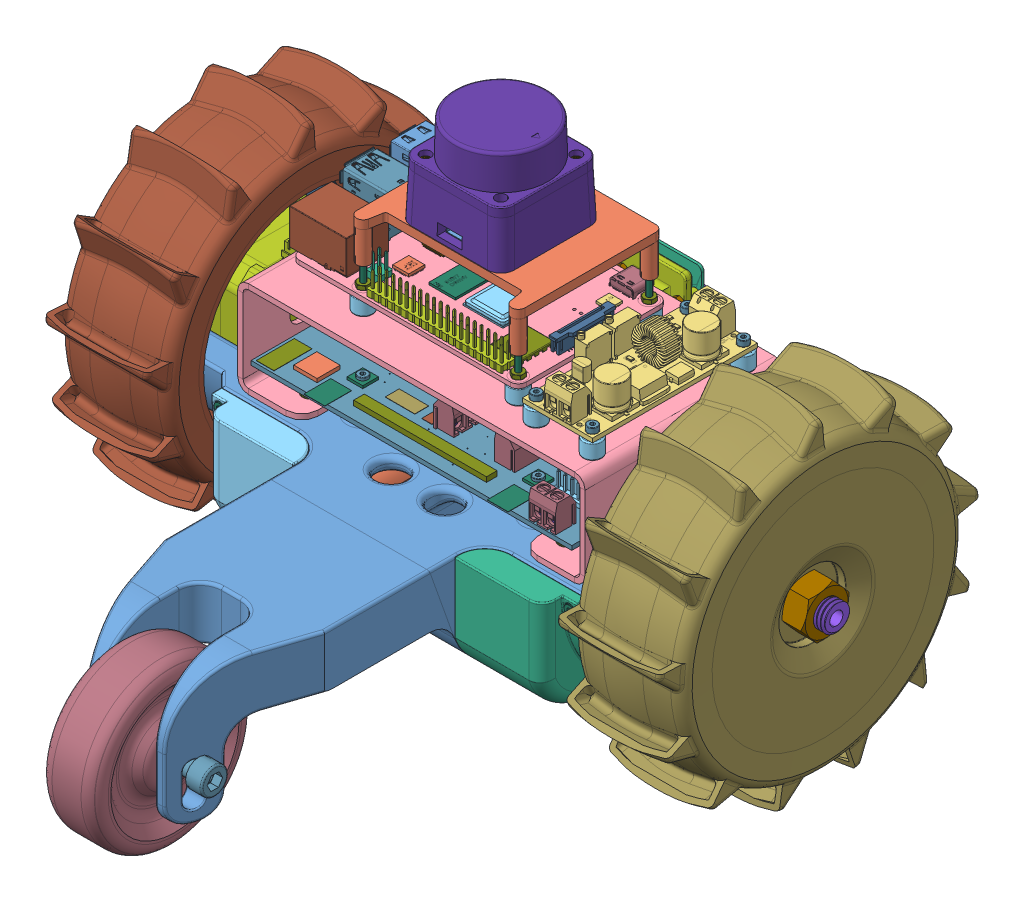
SolidWorks assembly RILey_assembly, configuration Default. Lengths in mm. (continued)
Mates (geometry in assembly coordinates): (continued)
- Width3: width aligned: plane of CameraMountBase-1 through (-15 21.3863 -20.622) normal (-1 0 0); plane of MiddlepartV1-1 through (15 21.3863 -20.622) normal (1 0 0); plane of CameraMountBase-1 through (61.5 -5 45) normal (-1 0 0); plane of MiddlepartV1-1 through (-61.5 -5 45) normal (1 0 0)
- Coincident33: coincident aligned: plane of DRV 8825 With Headers Assem-2/PCB-1 through (-15.9139 22.4151 10.2324) normal (0 1 0); plane of GY-91_MPU9250+BMP280 - Pins Down-1/GY-91 Base-1 through (23.0777 22.4151 10.2748) normal (0 1 0)
- Concentric20: concentric anti-aligned: cylinder of MiddlepartV1-1 through (-106.8137 0 0) axis (1 0 0) radius 4; cylinder of Nema 17_Slim-1 through (113.5 0 0) axis (-1 0 0) radius 2.5
- Concentric21: concentric anti-aligned: cylinder of socket head cap screw 4762_din-9 through (135.25 15.5 15.5) axis (1 0 0) radius 1.5; cylinder of Nema 17_Slim-1 through (95.5 15.5 15.5) axis (-1 0 0) radius 1.2645
- Coincident35: coincident anti-aligned: plane of MiddlepartV1-1 through (95.5 40 -40) normal (-1 0 0); plane of Nema 17_Slim-1 through (95.5 0 0) normal (1 0 0)
- Concentric22: concentric anti-aligned: cylinder of MiddlepartV1-1 through (-84.1863 0 0) axis (-1 0 0) radius 4; cylinder of Nema 17_Slim-2 through (-113.5 0 0) axis (1 0 0) radius 2.5
- Concentric23: concentric anti-aligned: cylinder of socket head cap screw 4762_din-3 through (-135.25 15.5 -15.5) axis (-1 0 0) radius 1.5; cylinder of Nema 17_Slim-2 through (-95.5 15.5 -15.5) axis (1 0 0) radius 1.2645
- Coincident36: coincident anti-aligned: plane of MiddlepartV1-1 through (-95.5 40 -40) normal (1 0 0); plane of Nema 17_Slim-2 through (-95.5 0 0) normal (-1 0 0)
- Distance1: distance = 155 mm anti-aligned: plane of wiel-1 through (75.1265 0 0) normal (-1 0 0); plane of wiel-2 through (71.8138 0 0) normal (-1 0 0)
- Concentric24: concentric anti-aligned: cylinder of wiel-1 through (85.7417 0 0) axis (1 0 0) radius 6.5; cylinder of Nema 17_Slim-1 through (113.5 0 0) axis (-1 0 0) radius 2.5
- Tangent5: tangent aligned: cylinder of MiddlepartV1-1 through (100.5 0 0) axis (-1 0 0) radius 40; plane of CameraMountBase-1 through (15 21.3863 -30) normal (0 0 -1)
- Tangent8: tangent anti-aligned: cylinder of 3_battery_pack-2/Li-ion Battery-1 through (14 -23 -26.7134) axis (0 0 -1) radius 9; plane of MiddlepartV1-1 through (-61.5 -32 45) normal (0 1 0)
- Width4: width anti-aligned: plane of MiddlepartV1-1 through (-2 0 0) normal (-1 0 0); plane of TimeOfFlightMount-1 through (2 0 0) normal (1 0 0); plane of MiddlepartV1-1 through (-5 -10.7713 -54.3331) normal (-0.984808 0.082851 0.152609); plane of TimeOfFlightMount-1 through (5 -10.7713 -54.3331) normal (0.984808 0.082851 0.152609)
- Coincident44: coincident anti-aligned: plane of MiddlepartV1-1 through (0 0 0) normal (0 1 0); plane of 3thFloor-1 through (0 0 0) normal (0 -1 0)
- Concentric31: concentric aligned: cylinder of MiddlepartV1-1 through (48 -9.9497 -27.5) axis (0 1 0) radius 1.75; cylinder of 3thFloor-1 through (48 -4.9497 -27.5) axis (0 1 0) radius 1.75
- Concentric32: concentric aligned: cylinder of MiddlepartV1-1 through (-48 -9.9497 -27.5) axis (0 1 0) radius 1.75; cylinder of 3thFloor-1 through (-48 -4.9497 -27.5) axis (0 1 0) radius 1.75
- Concentric37: concentric aligned: cylinder of 3thFloor-1 through (48 -4.9497 -27.5) axis (0 1 0) radius 1.75; cylinder of socket head cap screw 4762_din-11 through (48 37.75 -27.5) axis (0 1 0) radius 2.75
- Coincident47: coincident anti-aligned: plane of 3thFloor-1 through (41 3 37.5) normal (0 1 0); plane of socket head cap screw 4762_din-11 through (50.75 3 -27.5) normal (0 -1 0)
- Concentric38: concentric aligned: cylinder of 3thFloor-1 through (48 -4.9497 27.5) axis (0 1 0) radius 1.75; cylinder of socket head cap screw 4762_din-12 through (48 37.75 27.5) axis (0 1 0) radius 2.75
- Coincident48: coincident anti-aligned: plane of 3thFloor-1 through (41 3 37.5) normal (0 1 0); plane of socket head cap screw 4762_din-12 through (50.75 3 27.5) normal (0 -1 0)
- Concentric39: concentric aligned: cylinder of 3thFloor-1 through (-48 -4.9497 -27.5) axis (0 1 0) radius 1.75; cylinder of socket head cap screw 4762_din-13 through (-48 37.75 -27.5) axis (0 1 0) radius 2.75
- Coincident49: coincident anti-aligned: plane of 3thFloor-1 through (-41 3 37.5) normal (0 1 0); plane of socket head cap screw 4762_din-13 through (-45.25 3 -27.5) normal (0 -1 0)
- Concentric40: concentric aligned: cylinder of 3thFloor-1 through (-48 -4.9497 27.5) axis (0 1 0) radius 1.75; cylinder of socket head cap screw 4762_din-14 through (-48 37.75 27.5) axis (0 1 0) radius 2.75
- Coincident50: coincident anti-aligned: plane of 3thFloor-1 through (-41 3 37.5) normal (0 1 0); plane of socket head cap screw 4762_din-14 through (-45.25 3 27.5) normal (0 -1 0)
- Concentric41: concentric aligned: cylinder of socket head cap screw 4762_din-12 through (48 37.75 27.5) axis (0 1 0) radius 1.5; cylinder of hex nut style 1 gradeab_din-2 through (48 -30.234 27.5) axis (0 1 0) radius 1.5
- Concentric42: concentric anti-aligned: cylinder of MiddlepartV1-1 through (48 -9.9497 -27.5) axis (0 1 0) radius 1.75; cylinder of hex nut style 1 gradeab_din-3 through (48 17.6375 -27.5) axis (0 -1 0) radius 1.5
- Coincident51: coincident anti-aligned: plane of MiddlepartV1-1 through (-61.5 -5 45) normal (0 -1 0); plane of hex nut style 1 gradeab_din-3 through (48 -5 -24.3246) normal (0 1 0)
- Concentric43: concentric anti-aligned: cylinder of MiddlepartV1-1 through (-48 -9.9497 27.5) axis (0 1 0) radius 1.75; cylinder of hex nut style 1 gradeab_din-4 through (-48 17.6375 27.5) axis (0 -1 0) radius 1.5
- Coincident52: coincident anti-aligned: plane of MiddlepartV1-1 through (-61.5 -5 45) normal (0 -1 0); plane of hex nut style 1 gradeab_din-4 through (-48 -5 30.6754) normal (0 1 0)
- Concentric44: concentric anti-aligned: cylinder of MiddlepartV1-1 through (-48 -9.9497 -27.5) axis (0 1 0) radius 1.75; cylinder of hex nut style 1 gradeab_din-5 through (-48 17.6375 -27.5) axis (0 -1 0) radius 1.5
- Coincident53: coincident anti-aligned: plane of MiddlepartV1-1 through (-61.5 -5 45) normal (0 -1 0); plane of hex nut style 1 gradeab_din-5 through (-48 -5 -24.3246) normal (0 1 0)
- Concentric47: concentric aligned: cylinder of wiel-1 through (116.1265 0 0) axis (-1 0 0) radius 55.5; cylinder of socket head cap screw 4762_din-16 through (61.9923 0 0) axis (-1 0 0) radius 1.9
- Concentric59: concentric anti-aligned: cylinder of Nema 17_Slim-2 through (-113.5 0 0) axis (1 0 0) radius 2.5; cylinder of ReelyBuggyWheel-1 through (-163.278 0 0) axis (-1 0 0) radius 5.75
- Concentric60: concentric anti-aligned: cylinder of Nema 17_Slim-1 through (113.5 0 0) axis (-1 0 0) radius 2.5; cylinder of wiel-2 through (82.429 0 0) axis (1 0 0) radius 6.5
- Concentric61: concentric anti-aligned: cylinder of Nema 17_Slim-1 through (113.5 0 0) axis (-1 0 0) radius 2.5; cylinder of ReelyBuggyWheel_Left-1 through (106.7689 0 0) axis (1 0 0) radius 5.75
- Concentric62: concentric anti-aligned: cylinder of Nema 17_Slim-2 through (-113.5 0 0) axis (1 0 0) radius 2.5; cylinder of ReelyBuggyWheel_Right-1 through (-106.7689 0 0) axis (-1 0 0) radius 5.75
- Distance2: distance = 155 mm anti-aligned: cone of ReelyBuggyWheel_Left-1 through (75.7689 0 0) axis (1 0 0); cone of ReelyBuggyWheel_Right-1 through (-75.7689 0 0) axis (-1 0 0)
- Width7: width aligned: plane of ReelyBuggyWheel_Left-1 through (102.2689 0 0) normal (-1 0 0); plane of ReelyBuggyWheel_Right-1 through (-102.2689 0 0) normal (1 0 0); plane of MiddlepartV1-1 through (-100.5 0 0) normal (-1 0 0); plane of MiddlepartV1-1 through (100.5 0 0) normal (1 0 0)
- Concentric63: concentric anti-aligned: cylinder of Nema 17_Slim-2 through (-113.5 0 0) axis (1 0 0) radius 2.5; cylinder of ReelyBuggyWheel_Left-2 through (-106.5 0 0) axis (-1 0 0) radius 5.75
- Concentric64: concentric anti-aligned: cylinder of Nema 17_Slim-1 through (113.5 0 0) axis (-1 0 0) radius 2.5; cylinder of ReelyBuggyWheel_Right-2 through (106.5 0 0) axis (1 0 0) radius 5.75
- Concentric65: concentric aligned: cylinder of CameraMount-1 through (-8.25 3.5 -37) axis (1 0 0) radius 1.75; cylinder of socket head cap screw 4762_din-29 through (38.75 3.5 -37) axis (1 0 0) radius 1.9
- Coincident65: coincident anti-aligned: plane of CameraMount-1 through (5 4.049 -57.0786) normal (1 0 0); plane of socket head cap screw 4762_din-29 through (5 2.7745 -35.244) normal (-1 0 0)
- Concentric66: concentric aligned: cylinder of MiddlepartV1-1 through (-5.2527 -1 -43.5) axis (1 0 0) radius 1.15; cylinder of socket head cap screw 4762_din-30 through (38.75 -1 -43.5) axis (1 0 0) radius 1.9
- Concentric68: concentric anti-aligned: cylinder of socket head cap screw 4762_din-30 through (38.75 -1 -43.5) axis (1 0 0) radius 1; cylinder of hex nut style 1 gradeab_din-8 through (18.4375 -1 -43.5) axis (-1 0 0) radius 1
- Concentric71: concentric aligned: cylinder of 3thFloor-1 through (-31 45 -24.5) axis (0 -1 0) radius 1; cylinder of socket head cap screw 4762_din-35 through (-31 1.25 -24.5) axis (0 -1 0) radius 1.9
- Coincident71: coincident anti-aligned: plane of 3thFloor-1 through (0 35 0) normal (0 -1 0); plane of socket head cap screw 4762_din-35 through (-32.9 35 -24.5) normal (0 1 0)
- Concentric72: concentric aligned: cylinder of 3thFloor-1 through (-31 45 24.5) axis (0 -1 0) radius 1; cylinder of socket head cap screw 4762_din-36 through (-31 1.25 24.5) axis (0 -1 0) radius 1.9
- Coincident72: coincident anti-aligned: plane of 3thFloor-1 through (0 35 0) normal (0 -1 0); plane of socket head cap screw 4762_din-36 through (-32.9 35 24.5) normal (0 1 0)
- Concentric73: concentric aligned: cylinder of 3thFloor-1 through (27 45 -24.5) axis (0 -1 0) radius 1; cylinder of socket head cap screw 4762_din-37 through (27 1.25 -24.5) axis (0 -1 0) radius 1.9
- Coincident73: coincident anti-aligned: plane of 3thFloor-1 through (0 35 0) normal (0 -1 0); plane of socket head cap screw 4762_din-37 through (25.1 35 -24.5) normal (0 1 0)
- Concentric74: concentric aligned: cylinder of 3thFloor-1 through (27 45 24.5) axis (0 -1 0) radius 1; cylinder of socket head cap screw 4762_din-38 through (27 1.25 24.5) axis (0 -1 0) radius 1.9
- Coincident74: coincident anti-aligned: plane of 3thFloor-1 through (0 35 0) normal (0 -1 0); plane of socket head cap screw 4762_din-38 through (25.1 35 24.5) normal (0 1 0)
- Concentric75: concentric anti-aligned: cylinder of MiddlepartV1-1 through (-5.2527 3.5 -37) axis (1 0 0) radius 1.15; cylinder of CameraMount-1 through (5 3.5 -37) axis (-1 0 0) radius 1
- Coincident75: coincident anti-aligned: plane of Cam V2.1 v1.step-1 through (0 17.1066 -58.9285) normal (0 0.064849 0.997895); plane of CameraMount-1 through (-10.5 19.6013 -59.0906) normal (0 -0.064849 -0.997895)
- Width10: width anti-aligned: plane of CameraMount-1 through (2.25 1.6736 -18.8433) normal (-1 0 0); plane of MiddlepartV1-1 through (-2.25 1.6736 -18.8433) normal (1 0 0); plane of CameraMount-1 through (2 0 0) normal (1 0 0); plane of MiddlepartV1-1 through (-2 0 0) normal (-1 0 0)
- Concentric78: concentric aligned: cylinder of Cam V2.1 v1.step-1 through (10.5 7.1277 -58.28) axis (0 -0.064849 -0.997895) radius 1; cylinder of CameraMount-1 through (10.5 7.9707 -45.3074) axis (0 -0.064849 -0.997895) radius 1.25
- Concentric79: concentric aligned: cylinder of Cam V2.1 v1.step-1 through (-10.5 7.1277 -58.28) axis (0 -0.064849 -0.997895) radius 1; cylinder of CameraMount-1 through (-10.5 7.9707 -45.3074) axis (0 -0.064849 -0.997895) radius 1.25
- Width11: width anti-aligned: plane of Backwheel-1 through (-10.5 -32.6496 136.5106) normal (-1 0 0); plane of MiddlepartV1-2 through (10.5 -32.6496 136.5106) normal (1 0 0); plane of Backwheel-1 through (-11.5 0 105) normal (1 0 0); plane of MiddlepartV1-2 through (11.5 0 105) normal (-1 0 0)
- Tangent10: tangent aligned: cylinder of MiddlepartV1-2 through (35.6484 -32.5 136.5) axis (-1 0 0) radius 3.1; cylinder of Backwheel-1 through (-10.5 -32.6496 136.5106) axis (1 0 0) radius 3.25
- Concentric102: concentric aligned: cylinder of Cam V2.1 v1.step-1 through (-10.5 19.6013 -59.0906) axis (0 -0.064849 -0.997895) radius 1; cylinder of socket head cap screw 4762_din-51 through (-10.5 17.3479 -93.7675) axis (0 -0.064849 -0.997895) radius 1.9
- Coincident99: coincident anti-aligned: plane of Cam V2.1 v1.step-1 through (0 17.0418 -59.9264) normal (0 -0.064849 -0.997895); plane of socket head cap screw 4762_din-51 through (-10.6232 21.4285 -60.2115) normal (0 0.064849 0.997895)
- Concentric103: concentric aligned: cylinder of Cam V2.1 v1.step-1 through (-10.5 7.1277 -58.28) axis (0 -0.064849 -0.997895) radius 1; cylinder of socket head cap screw 4762_din-52 through (-10.5 4.8742 -92.9569) axis (0 -0.064849 -0.997895) radius 1.9
- Coincident100: coincident anti-aligned: plane of Cam V2.1 v1.step-1 through (0 17.0418 -59.9264) normal (0 -0.064849 -0.997895); plane of socket head cap screw 4762_din-52 through (-10.6232 8.9548 -59.4009) normal (0 0.064849 0.997895)
- Concentric104: concentric aligned: cylinder of Cam V2.1 v1.step-1 through (10.5 7.1277 -58.28) axis (0 -0.064849 -0.997895) radius 1; cylinder of socket head cap screw 4762_din-53 through (10.5 4.8742 -92.9569) axis (0 -0.064849 -0.997895) radius 1.9
- Coincident101: coincident anti-aligned: plane of Cam V2.1 v1.step-1 through (0 17.0418 -59.9264) normal (0 -0.064849 -0.997895); plane of socket head cap screw 4762_din-53 through (10.3768 8.9548 -59.4009) normal (0 0.064849 0.997895)
- Concentric105: concentric aligned: cylinder of Cam V2.1 v1.step-1 through (10.5 19.6013 -59.0906) axis (0 -0.064849 -0.997895) radius 1; cylinder of socket head cap screw 4762_din-54 through (10.5 17.3479 -93.7675) axis (0 -0.064849 -0.997895) radius 1.9
- Coincident102: coincident anti-aligned: plane of Cam V2.1 v1.step-1 through (0 17.0418 -59.9264) normal (0 -0.064849 -0.997895); plane of socket head cap screw 4762_din-54 through (10.3768 21.4285 -60.2115) normal (0 0.064849 0.997895)
- Concentric108: concentric anti-aligned: cylinder of MiddlepartV1-1 through (48 -9.9497 -27.5) axis (0 1 0) radius 1.75; cylinder of socket head cap screw 4762_din-58 through (48 -39.75 -27.5) axis (0 -1 0) radius 2.75
- Coincident105: coincident anti-aligned: plane of MiddlepartV1-1 through (-61.5 -5 45) normal (0 -1 0); plane of socket head cap screw 4762_din-58 through (45.25 -5 -27.5) normal (0 1 0)
- Concentric109: concentric anti-aligned: cylinder of MiddlepartV1-1 through (-48 -9.9497 -27.5) axis (0 1 0) radius 1.75; cylinder of socket head cap screw 4762_din-59 through (-48 -39.75 -27.5) axis (0 -1 0) radius 2.75
- Coincident106: coincident anti-aligned: plane of MiddlepartV1-1 through (-61.5 -5 45) normal (0 -1 0); plane of socket head cap screw 4762_din-59 through (-50.75 -5 -27.5) normal (0 1 0)
- Concentric110: concentric anti-aligned: cylinder of MiddlepartV1-1 through (-48 -9.9497 27.5) axis (0 1 0) radius 1.75; cylinder of socket head cap screw 4762_din-61 through (-48 -39.75 27.5) axis (0 -1 0) radius 2.75
- Coincident107: coincident anti-aligned: plane of MiddlepartV1-1 through (-61.5 -5 45) normal (0 -1 0); plane of socket head cap screw 4762_din-61 through (-50.75 -5 27.5) normal (0 1 0)
- Concentric111: concentric anti-aligned: cylinder of MiddlepartV1-1 through (48 -9.9497 27.5) axis (0 1 0) radius 1.75; cylinder of socket head cap screw 4762_din-62 through (48 -39.75 27.5) axis (0 -1 0) radius 2.75
- Coincident108: coincident anti-aligned: plane of MiddlepartV1-1 through (-61.5 -5 45) normal (0 -1 0); plane of socket head cap screw 4762_din-62 through (45.25 -5 27.5) normal (0 1 0)
- Concentric120: concentric: cylinder of Backwheel-1 through (-10.5 -32.6496 136.5106) axis (1 0 0) radius 3.25; cylinder of socket head cap screw 4762_din-64 through (-64.9282 -39.2304 114.5914) axis (-0.948683 0 0.316228) radius 5
- Concentric1211: concentric aligned: cylinder of Backwheel-1 through (-10.5 -32.6496 136.5106) axis (1 0 0) radius 3.25; cylinder of socket head cap screw 4762_din-66 through (57.2465 -32.6496 136.5106) axis (1 0 0) radius 5
- Tangent152: tangent: plane of MiddlepartV1-2 through (30 -97.4342 100) normal (0.948683 0 0.316228); circle of socket head cap screw 4762_din-66
- Concentric122: concentric aligned: cone of socket head cap screw 4762_din-66 through (-25.5035 -32.6496 136.5106) axis (-1 0 0); cylinder of hex nut style 1 gradeab_din-20 through (0.8569 -39.2304 136.65) axis (-1 0 0) radius 3
- Coincident122: coincident: line of MiddlepartV1-1 through (-18.9806 -42.5 133.0581) axis (0 1 0); plane of hex nut style 1 gradeab_din-20 through (-18.9806 -39.2304 126.65) normal (1 0 0)
- Concentric1214: concentric aligned: cylinder of ReelyBuggyWheel_Right-2 through (106.5 0 0) axis (1 0 0) radius 5.75; cylinder of hex nut style 1 gradeab_iso-2 through (92.8625 0 0) axis (1 0 0) radius 5
- Coincident131: coincident anti-aligned: plane of ReelyBuggyWheel_Right-2 through (109.5 0 0) normal (1 0 0); plane of hex nut style 1 gradeab_iso-2 through (109.5 0 16) normal (-1 0 0)
- Concentric1215: concentric aligned: cylinder of ReelyBuggyWheel_Left-2 through (-106.5 0 0) axis (-1 0 0) radius 5.75; cylinder of hex nut style 1 gradeab_iso-3 through (-92.8625 0 0) axis (-1 0 0) radius 5
- Coincident132: coincident anti-aligned: plane of ReelyBuggyWheel_Left-2 through (-109.5 0 0) normal (-1 0 0); plane of hex nut style 1 gradeab_iso-3 through (-109.5 -2.0616 -15.8666) normal (1 0 0)
- Width12: width aligned: plane of 3_battery_pack-1/link2-2 through (-10 -24.5 -26.9134) normal (1 0 0); plane of MiddlepartV1-1 through (-54 -21.5 -26.9134) normal (-1 0 0); plane of 3_battery_pack-1/link2-2 through (-61.5 -5 45) normal (1 0 0); plane of MiddlepartV1-1 through (-2.5 0 0) normal (-1 0 0)
- Tangent12: tangent anti-aligned: plane of MiddlepartV1-1 through (-61.5 -32 45) normal (0 1 0); cylinder of 3_battery_pack-2/Li-ion Battery-3 through (50 -23 -26.7134) axis (0 0 -1) radius 9
- Coincident138: coincident aligned: plane of 3_battery_pack-1/link2-2 through (-11 -24.5 -26.9134) normal (0 0 -1); plane of 3_battery_pack-2/link2-2 through (53 -24.5 -26.9134) normal (0 0 -1)
- Width13: width anti-aligned: plane of 3_battery_pack-2/link2-2 through (10 -21.5 -26.9134) normal (-1 0 0); plane of 3_battery_pack-2/link2-2 through (54 -24.5 -26.9134) normal (1 0 0); plane of MiddlepartV1-1 through (2.5 0 0) normal (1 0 0); plane of MiddlepartV1-1 through (61.5 -5 45) normal (-1 0 0)
- Concentric1220: concentric aligned: cylinder of Nema 17_Slim-2 through (-113.5 0 0) axis (1 0 0) radius 2.5; cylinder of hex screw gradeab fine_iso-1 through (-100.5 0 0) axis (1 0 0) radius 5
- Coincident139: coincident anti-aligned: plane of MiddlepartV1-1 through (-100.5 0 0) normal (-1 0 0); plane of hex screw gradeab fine_iso-1 through (-100.5 -2.768 8.8132) normal (1 0 0)
- Parallel6: parallel anti-aligned: plane of ReelyBuggyWheel_Left-2 through (-106.5 8.4437 -4.875) normal (0 -1 0); plane of hex screw gradeab fine_iso-1 through (-106.9 6.2484 6.8037) normal (0 0.954052 0.299641)
- Coincident141: coincident anti-aligned: plane of ReelyBuggyWheel_Left-2 through (-106.5 0 0) normal (1 0 0); plane of hex screw gradeab fine_iso-1 through (-106.9 -2.768 8.8132) normal (-1 0 0)
- Coincident142: coincident anti-aligned: plane of MiddlepartV1-1 through (100.5 0 0) normal (1 0 0); plane of hex screw gradeab fine_iso-2 through (100.5 9.2376 0) normal (-1 0 0)
- Concentric1222: concentric aligned: cylinder of Nema 17_Slim-1 through (113.5 0 0) axis (-1 0 0) radius 2.5; cylinder of hex screw gradeab fine_iso-2 through (100.5 0 0) axis (-1 0 0) radius 5
- Parallel7: parallel anti-aligned: plane of ReelyBuggyWheel_Right-2 through (106.5 8.4437 4.875) normal (0 -1 0); plane of hex screw gradeab fine_iso-2 through (106.9 9.2376 0) normal (0 0.866025 0.5)
- Coincident144: coincident anti-aligned: plane of ReelyBuggyWheel_Right-2 through (106.5 0 0) normal (-1 0 0); plane of hex screw gradeab fine_iso-2 through (106.9 9.2376 0) normal (1 0 0)
- Concentric1224: concentric anti-aligned: cylinder of MiddlepartV1-1 through (100.5 0 0) axis (-1 0 0) radius 40; cylinder of BatteryCoverFront-1 through (-68.5 0 0) axis (1 0 0) radius 40
- Concentric1225: concentric aligned: cylinder of MiddlepartV1-1 through (-65.5 -3.5 -50) axis (0 0 1) radius 1; cylinder of BatteryCoverFront-1 through (-65.5 -3.5 -44) axis (0 0 1) radius 1
- Concentric1226: concentric aligned: cylinder of MiddlepartV1-1 through (65.5 -3.5 -50) axis (0 0 1) radius 1; cylinder of BatteryCoverFront-1 through (65.5 -3.5 -44) axis (0 0 1) radius 1
- Concentric1229: concentric anti-aligned: cylinder of MiddlepartV1-1 through (65.5 -3.5 -50) axis (0 0 1) radius 1; cylinder of socket head cap screw_iso-9 through (65.5 -3.5 -75.75) axis (0 0 -1) radius 1
- Concentric1231: concentric anti-aligned: cylinder of MiddlepartV1-1 through (-65.5 -3.5 -50) axis (0 0 1) radius 1; cylinder of socket head cap screw_iso-13 through (-65.5 -3.5 -75.75) axis (0 0 -1) radius 1
- Concentric1232: concentric anti-aligned: cylinder of MiddlepartV1-1 through (-65.5 -36.5 -25) axis (0 0 1) radius 1; cylinder of socket head cap screw_iso-15 through (-65.5 -36.5 -55.75) axis (0 0 -1) radius 1
- Concentric1233: concentric anti-aligned: cylinder of MiddlepartV1-1 through (0 -36.5 -25) axis (0 0 1) radius 1; cylinder of socket head cap screw_iso-17 through (0 -36.5 -55.75) axis (0 0 -1) radius 1
- Concentric1234: concentric anti-aligned: cylinder of MiddlepartV1-1 through (65.5 -36.5 -25) axis (0 0 1) radius 1; cylinder of socket head cap screw_iso-16 through (65.5 -36.5 -55.75) axis (0 0 -1) radius 1
- Concentric1246: concentric anti-aligned: cylinder of MiddlepartV1-1 through (-32.85 10 22.85) axis (0 -1 0) radius 1; cylinder of RILey_PCB-1/RILey_PCB.step-1/PCB Component.step-1/Board.step-1 through (-32.85 10 22.85) axis (0 1 0) radius 1.4
- Concentric1248: concentric anti-aligned: cylinder of MiddlepartV1-1 through (32.85 10 -22.85) axis (0 -1 0) radius 1; cylinder of RILey_PCB-1/RILey_PCB.step-1/PCB Component.step-1/Board.step-1 through (32.85 10 -22.85) axis (0 1 0) radius 1.4
- Coincident152: coincident anti-aligned: plane of MiddlepartV1-1 through (32.85 10 -22.85) normal (0 1 0); plane of RILey_PCB-1/RILey_PCB.step-1/PCB Component.step-1/Board.step-1 through (0 10 2.5) normal (0 -1 0)
- Concentric1249: concentric anti-aligned: circle of MiddlepartV1-1; cylinder of socket head cap screw 4762_din-25 through (32.85 45.32 -22.85) axis (0 1 0) radius 1
- Concentric1250: concentric anti-aligned: circle of MiddlepartV1-1; cylinder of socket head cap screw 4762_din-26 through (32.85 45.32 22.85) axis (0 1 0) radius 1
- Concentric1251: concentric anti-aligned: circle of MiddlepartV1-1; cylinder of socket head cap screw 4762_din-27 through (-32.85 45.32 22.85) axis (0 1 0) radius 1
- Concentric1252: concentric anti-aligned: circle of MiddlepartV1-1; cylinder of socket head cap screw 4762_din-22 through (-32.85 45.32 -22.85) axis (0 1 0) radius 1
- Coincident157: coincident anti-aligned: plane of socket head cap screw 4762_din-27 through (-30.95 11.57 22.85) normal (0 -1 0); plane of RILey_PCB-1/RILey_PCB.step-1/PCB Component.step-1/Board.step-1 through (0 11.57 2.5) normal (0 1 0)
- Coincident158: coincident anti-aligned: plane of socket head cap screw 4762_din-26 through (34.75 11.57 22.85) normal (0 -1 0); plane of RILey_PCB-1/RILey_PCB.step-1/PCB Component.step-1/Board.step-1 through (0 11.57 2.5) normal (0 1 0)
- Coincident159: coincident anti-aligned: plane of socket head cap screw 4762_din-25 through (34.75 11.57 -22.85) normal (0 -1 0); plane of RILey_PCB-1/RILey_PCB.step-1/PCB Component.step-1/Board.step-1 through (0 11.57 2.5) normal (0 1 0)
- Coincident160: coincident anti-aligned: plane of socket head cap screw 4762_din-22 through (-30.95 11.57 -22.85) normal (0 -1 0); plane of RILey_PCB-1/RILey_PCB.step-1/PCB Component.step-1/Board.step-1 through (0 11.57 2.5) normal (0 1 0)
- Concentric1253: concentric aligned: cylinder of MiddlepartV1-1 through (65.5 -3.5 50) axis (0 0 -1) radius 1; cylinder of BatteryCoverBackRight-1 through (65.5 -3.5 51.5671) axis (0 0 -1) radius 1
- Concentric1254: concentric aligned: cylinder of MiddlepartV1-1 through (65.5 -36.5 25) axis (0 0 -1) radius 1; cylinder of BatteryCoverBackRight-1 through (65.5 -36.5 51.5671) axis (0 0 -1) radius 1
- Concentric1255: concentric aligned: cylinder of MiddlepartV1-1 through (-65.5 -3.5 50) axis (0 0 -1) radius 1; cylinder of BatteryCoverBackLeft-1 through (-65.5 -3.5 51.5671) axis (0 0 -1) radius 1
- Concentric1256: concentric aligned: cylinder of MiddlepartV1-1 through (-65.5 -36.5 25) axis (0 0 -1) radius 1; cylinder of BatteryCoverBackLeft-1 through (-65.5 -36.5 51.5671) axis (0 0 -1) radius 1
- Concentric1257: concentric aligned: cylinder of MiddlepartV1-1 through (100.5 0 0) axis (-1 0 0) radius 40; cylinder of BatteryCoverBackLeft-1 through (-30 0 0) axis (-1 0 0) radius 40
- Concentric1258: concentric aligned: cylinder of MiddlepartV1-1 through (100.5 0 0) axis (-1 0 0) radius 40; cylinder of BatteryCoverBackRight-1 through (30 0 0) axis (-1 0 0) radius 40
- Concentric1259: concentric aligned: cylinder of BatteryCoverBackRight-1 through (65.5 -36.5 23.0671) axis (0 0 1) radius 2; cylinder of socket head cap screw_iso-19 through (65.5 -36.5 56.8171) axis (0 0 1) radius 1.9
- Coincident161: coincident anti-aligned: plane of BatteryCoverBackRight-1 through (65.5 -36.5 23.0671) normal (0 0 1); plane of socket head cap screw_iso-19 through (65.5 -34.6 23.0671) normal (0 0 -1)
- Concentric1260: concentric aligned: cylinder of BatteryCoverBackLeft-1 through (-65.5 -36.5 23.0671) axis (0 0 1) radius 2; cylinder of socket head cap screw_iso-20 through (-65.5 -36.5 56.8171) axis (0 0 1) radius 1.9
- Coincident162: coincident anti-aligned: plane of BatteryCoverBackLeft-1 through (-65.5 -36.5 23.0671) normal (0 0 1); plane of socket head cap screw_iso-20 through (-65.5 -34.6 23.0671) normal (0 0 -1)
- Concentric1261: concentric aligned: cylinder of BatteryCoverBackRight-1 through (65.5 -3.5 42.0671) axis (0 0 1) radius 2; cylinder of socket head cap screw_iso-22 through (65.5 -3.5 75.8171) axis (0 0 1) radius 1.9
- Coincident163: coincident anti-aligned: plane of BatteryCoverBackRight-1 through (65.5 -3.5 42.0671) normal (0 0 1); plane of socket head cap screw_iso-22 through (65.5 -1.6 42.0671) normal (0 0 -1)
- Concentric1262: concentric aligned: cylinder of BatteryCoverBackLeft-1 through (-65.5 -3.5 42.0671) axis (0 0 1) radius 2; cylinder of socket head cap screw_iso-23 through (-65.5 -3.5 75.8171) axis (0 0 1) radius 1.9
- Coincident164: coincident anti-aligned: plane of BatteryCoverBackLeft-1 through (-65.5 -3.5 42.0671) normal (0 0 1); plane of socket head cap screw_iso-23 through (-65.5 -1.6 42.0671) normal (0 0 -1)
- Coincident166: coincident anti-aligned: plane of BatteryCoverFront-1 through (65.5 -3.5 -42) normal (0 0 -1); plane of socket head cap screw_iso-9 through (66.9813 -2.3101 -42) normal (0 0 1)
- Coincident167: coincident anti-aligned: plane of BatteryCoverFront-1 through (65.5 -36.5 -22) normal (0 0 -1); plane of socket head cap screw_iso-16 through (64.3101 -35.0187 -22) normal (0 0 1)
- Coincident168: coincident anti-aligned: plane of BatteryCoverFront-1 through (0 -36.5 -22) normal (0 0 -1); plane of socket head cap screw_iso-17 through (0.6879 -34.7289 -22) normal (0 0 1)
- Coincident169: coincident anti-aligned: plane of BatteryCoverFront-1 through (-65.5 -36.5 -22) normal (0 0 -1); plane of socket head cap screw_iso-15 through (-63.8683 -37.4734 -22) normal (0 0 1)
- Coincident170: coincident anti-aligned: plane of BatteryCoverFront-1 through (-65.5 -3.5 -42) normal (0 0 -1); plane of socket head cap screw_iso-13 through (-66.0001 -5.333 -42) normal (0 0 1)
- Coincident173: coincident anti-aligned: plane of RILey_PCB-1/RILey_PCB.step-1/PCB Component.step-1/Board.step-1 through (0 11.57 2.5) normal (0 1 0); plane of DG301-5.0-02-1 through (38.33 11.57 29.74) normal (0 -1 0)
- Coincident182: coincident anti-aligned: plane of MiddlepartV1-1 through (-100.5 0 0) normal (-1 0 0); plane of HexBolt_modified-1 through (-100.5 0 0) normal (1 0 0)
- Concentric1271: concentric aligned: cylinder of Nema 17_Slim-2 through (-113.5 0 0) axis (1 0 0) radius 2.5; cylinder of HexBolt_modified-1 through (-128.5711 0 0) axis (1 0 0) radius 2.5
- Parallel8: parallel aligned: plane of Nema 17_Slim-2 through (-122.5 2 1.5) normal (0 1 0); plane of HexBolt_modified-1 through (-106.5 8.5 4.9075) normal (0 1 0)
- Concentric1272: concentric anti-aligned: cylinder of ReelyBuggyWheel_Left-2 through (-106.5 0 0) axis (-1 0 0) radius 5.75; cylinder of HexBolt_modified-1 through (-128.5711 0 0) axis (1 0 0) radius 2.5
- Parallel9: parallel anti-aligned: plane of ReelyBuggyWheel_Left-2 through (-106.5 8.4437 -4.875) normal (0 -1 0); plane of HexBolt_modified-1 through (-106.5 8.5 4.9075) normal (0 1 0)
- Coincident185: coincident anti-aligned: plane of ReelyBuggyWheel_Left-2 through (-106.5 0 0) normal (1 0 0); plane of HexBolt_modified-1 through (-106.5 0 0) normal (-1 0 0)
- Coincident186: coincident anti-aligned: plane of MiddlepartV1-1 through (100.5 0 0) normal (1 0 0); plane of HexBolt_modified-2 through (100.5 0 0) normal (-1 0 0)
- Concentric1274: concentric aligned: cylinder of Nema 17_Slim-1 through (113.5 0 0) axis (-1 0 0) radius 2.5; cylinder of HexBolt_modified-2 through (128.5711 0 0) axis (-1 0 0) radius 2.5
- Parallel10: parallel aligned: plane of Nema 17_Slim-1 through (122.5 2 -1.5) normal (0 1 0); plane of HexBolt_modified-2 through (106.5 8.5 -4.9075) normal (0 1 0)
- Concentric1275: concentric anti-aligned: cylinder of ReelyBuggyWheel_Right-2 through (106.5 0 0) axis (1 0 0) radius 5.75; cylinder of HexBolt_modified-2 through (128.5711 0 0) axis (-1 0 0) radius 2.5
- Parallel11: parallel anti-aligned: plane of ReelyBuggyWheel_Right-2 through (106.5 8.4437 4.875) normal (0 -1 0); plane of HexBolt_modified-2 through (106.5 8.5 -4.9075) normal (0 1 0)
- Coincident189: coincident anti-aligned: plane of ReelyBuggyWheel_Right-2 through (106.5 0 0) normal (-1 0 0); plane of HexBolt_modified-2 through (106.5 0 0) normal (1 0 0)
- Concentric12821: concentric aligned: cylinder of MiddlepartV1-1 through (-5.2527 3.5 -37) axis (1 0 0) radius 1.15; cylinder of socket head cap screw 4762_din-32 through (38.75 3.5 -37) axis (1 0 0) radius 1
- Coincident1971: coincident anti-aligned: plane of CameraMount-1 through (5 5.3264 -55.1567) normal (1 0 0); plane of socket head cap screw 4762_din-32 through (5 2.3436 -35.4924) normal (-1 0 0)
- Coincident1981: coincident anti-aligned: plane of CameraMount-1 through (-5 5.3264 -55.1567) normal (-1 0 0); plane of hex nut style 1 gradeab_iso-16 through (-5 1.1349 -40.2259) normal (1 0 0)
- Concentric12831: concentric anti-aligned: cylinder of socket head cap screw 4762_din-32 through (38.75 3.5 -37) axis (1 0 0) radius 1; cylinder of hex nut style 1 gradeab_iso-16 through (-5 3.5 -37) axis (-1 0 0) radius 0.8
- Concentric1289: concentric aligned: cone of socket head cap screw 4762_din-66 through (-25.5035 -32.6496 136.5106) axis (-1 0 0); cylinder of hex nut style 1 gradeab_iso-26 through (0.341 -32.6496 136.5106) axis (-1 0 0) radius 3
- Tangent151: tangent: plane of MiddlepartV1-2 through (-30 -97.4342 100) normal (-0.948683 0 0.316228); circle of hex nut style 1 gradeab_iso-26
- Coincident1992: coincident anti-aligned: plane of MiddlepartV1-1 through (0 0 0) normal (0 1 0); plane of Assem2^RILey_assembly-1/3rdFloor_Sheetmetal-1 through (0 0 0) normal (0 -1 0)
- Concentric12832: concentric aligned: cylinder of MiddlepartV1-1 through (48 -9.9497 27.5) axis (0 1 0) radius 1.75; cylinder of Assem2^RILey_assembly-1/3rdFloor_Sheetmetal-1 through (48 -4.9497 27.5) axis (0 1 0) radius 1.75
- Concentric12833: concentric aligned: cylinder of MiddlepartV1-1 through (48 -9.9497 -27.5) axis (0 1 0) radius 1.75; cylinder of Assem2^RILey_assembly-1/3rdFloor_Sheetmetal-1 through (48 -4.9497 -27.5) axis (0 1 0) radius 1.75
- Concentric12834: concentric aligned: cylinder of Assem2^RILey_assembly-1/3rdFloor_Sheetmetal-1 through (48 -4.9497 27.5) axis (0 1 0) radius 1.75; cylinder of hex nut style 1 gradeab_iso-21 through (48 -20.6375 27.5) axis (0 1 0) radius 1.5
- Coincident1993: coincident anti-aligned: plane of Assem2^RILey_assembly-1/3rdFloor_Sheetmetal-1 through (0 2 0) normal (0 1 0); plane of hex nut style 1 gradeab_iso-21 through (48 2 24.3246) normal (0 -1 0)
- Concentric12835: concentric aligned: cylinder of Assem2^RILey_assembly-1/3rdFloor_Sheetmetal-1 through (-48 -4.9497 27.5) axis (0 1 0) radius 1.75; cylinder of hex nut style 1 gradeab_iso-22 through (-48 -20.6375 27.5) axis (0 1 0) radius 1.5
- Coincident1994: coincident anti-aligned: plane of Assem2^RILey_assembly-1/3rdFloor_Sheetmetal-1 through (0 2 0) normal (0 1 0); plane of hex nut style 1 gradeab_iso-22 through (-48 2 24.3246) normal (0 -1 0)
- Concentric12836: concentric aligned: cylinder of Assem2^RILey_assembly-1/3rdFloor_Sheetmetal-1 through (-48 -4.9497 -27.5) axis (0 1 0) radius 1.75; cylinder of hex nut style 1 gradeab_iso-23 through (-48 -20.6375 -27.5) axis (0 1 0) radius 1.5
- Coincident1995: coincident anti-aligned: plane of Assem2^RILey_assembly-1/3rdFloor_Sheetmetal-1 through (0 2 0) normal (0 1 0); plane of hex nut style 1 gradeab_iso-23 through (-48 2 -30.6754) normal (0 -1 0)
- Concentric12837: concentric aligned: cylinder of Assem2^RILey_assembly-1/3rdFloor_Sheetmetal-1 through (48 -4.9497 -27.5) axis (0 1 0) radius 1.75; cylinder of hex nut style 1 gradeab_iso-24 through (48 -20.6375 -27.5) axis (0 1 0) radius 1.5
- Coincident1996: coincident anti-aligned: plane of Assem2^RILey_assembly-1/3rdFloor_Sheetmetal-1 through (0 2 0) normal (0 1 0); plane of hex nut style 1 gradeab_iso-24 through (48 2 -30.6754) normal (0 -1 0)
- Concentric12838: concentric anti-aligned: cylinder of MiddlepartV1-1 through (-5.2527 3.5 -37) axis (1 0 0) radius 1.15; cylinder of CameraAssembly-1/CameraMount-1 through (5 3.5 -37) axis (-1 0 0) radius 1
- Width14: width aligned: plane of CameraAssembly-1/CameraMount-1 through (-5 6.1036 -55.0616) normal (-1 0 0); plane of CameraAssembly-1/CameraMount-1 through (5 6.1036 -55.0616) normal (1 0 0); plane of MiddlepartV1-1 through (-2 0 0) normal (-1 0 0); plane of MiddlepartV1-1 through (2 0 0) normal (1 0 0)
- Coincident1997: coincident anti-aligned: plane of socket head cap screw 4762_din-32 through (5 2.3436 -35.4924) normal (-1 0 0); plane of CameraAssembly-1/CameraMount-1 through (5 6.1036 -55.0616) normal (1 0 0)
- Coincident1999: coincident anti-aligned: plane of hex nut style 1 gradeab_iso-16 through (-5 1.1349 -40.2259) normal (1 0 0); plane of CameraAssembly-1/CameraMount-1 through (-5 6.1036 -55.0616) normal (-1 0 0)
- Width15: width aligned: plane of MiddlepartV1-1 through (-2 0 0) normal (-1 0 0); plane of MiddlepartV1-1 through (2 0 0) normal (1 0 0); plane of Assem33^RILey_assembly-1/TimeOfFlightMount-1; plane of Assem33^RILey_assembly-1/TimeOfFlightMount-1
- Concentric12839: concentric aligned: cylinder of MiddlepartV1-1 through (-5.2527 -1 -43.5) axis (1 0 0) radius 1.15; cylinder of Assem33^RILey_assembly-1/TimeOfFlightMount-1 through (8.2527 -1 -43.5) axis (-1 0 0) radius 1.15
- Concentric12840: concentric anti-aligned: cylinder of Assem33^RILey_assembly-1/TimeOfFlightMount-1 through (8.2527 -1 -43.5) axis (-1 0 0) radius 1.15; cylinder of socket head cap screw 4762_din-33 through (38.75 -1 -43.5) axis (1 0 0) radius 1.9
- Coincident2000: coincident anti-aligned: plane of Assem33^RILey_assembly-1/TimeOfFlightMount-1; plane of socket head cap screw 4762_din-33
- Coincident2001: coincident anti-aligned: plane of Assem33^RILey_assembly-1/TimeOfFlightMount-1 through (-5 -2.007 -40.1109) normal (-1 0 0); plane of hex nut style 1 gradeab_iso-11 through (-5 -3.1726 -46.8585) normal (1 0 0)
- Parallel121: parallel aligned: plane of Nema 17_Slim-2 through (-122.5 2 1.5) normal (0 1 0); plane of LeftWheelAssembly-1/HexBolt_modified-1 through (-106.5 8.5 4.9075) normal (0 1 0)
- Concentric128411: concentric aligned: cylinder of Nema 17_Slim-2 through (-113.5 0 0) axis (1 0 0) radius 2.5; cylinder of LeftWheelAssembly-1/HexBolt_modified-1 through (-128.5711 0 0) axis (1 0 0) radius 2.5
- Coincident20031: coincident anti-aligned: plane of MiddlepartV1-1 through (-100.5 0 0) normal (-1 0 0); plane of LeftWheelAssembly-1/HexBolt_modified-1 through (-100.5 0 0) normal (1 0 0)
- Parallel131: parallel aligned: plane of Nema 17_Slim-1 through (122.5 2 -1.5) normal (0 1 0); plane of RightWheelAssembly-1/HexBolt_modified-1 through (106.5 8.5 -4.9075) normal (0 1 0)
- Concentric128421: concentric aligned: cylinder of Nema 17_Slim-1 through (113.5 0 0) axis (-1 0 0) radius 2.5; cylinder of RightWheelAssembly-1/HexBolt_modified-1 through (128.5711 0 0) axis (-1 0 0) radius 2.5
- Coincident2005: coincident anti-aligned: plane of MiddlepartV1-1 through (100.5 0 0) normal (1 0 0); plane of RightWheelAssembly-1/HexBolt_modified-1 through (100.5 0 0) normal (-1 0 0)
- Concentric128422: concentric aligned: cylinder of MiddlepartV1-1 through (-19 -15 60.7843) axis (0 0 -1) radius 2.65; cylinder of MiddlepartV1-2 through (-19 -15 84.6855) axis (0 0 -1) radius 2.25
- Concentric128423: concentric aligned: cylinder of MiddlepartV1-1 through (19 -15 60.7843) axis (0 0 -1) radius 2.65; cylinder of MiddlepartV1-2 through (19 -15 84.6855) axis (0 0 -1) radius 2.25
- Coincident20032: coincident anti-aligned: plane of MiddlepartV1-1 through (0 -19.1027 54.0305) normal (0 -0.333333 0.942809); plane of MiddlepartV1-2 through (0 -19.1027 54.0305) normal (0 0.333333 -0.942809)
- Concentric128424: concentric aligned: cylinder of MiddlepartV1-1 through (-19 -15 49) axis (0 0 -1) radius 4.35; cylinder of socket head cap screw_iso-26 through (-19 -15 12.25) axis (0 0 -1) radius 4.25
- Coincident20033: coincident anti-aligned: plane of MiddlepartV1-1 through (-19 -15 49) normal (0 0 -1); plane of socket head cap screw_iso-26 through (-19 -10.75 49) normal (0 0 1)
- Concentric128425: concentric aligned: cylinder of MiddlepartV1-1 through (19 -15 49) axis (0 0 -1) radius 4.35; cylinder of socket head cap screw_iso-27 through (19 -15 12.25) axis (0 0 -1) radius 4.25
- Coincident20034: coincident anti-aligned: plane of MiddlepartV1-1 through (19 -15 49) normal (0 0 -1); plane of socket head cap screw_iso-27 through (19 -10.75 49) normal (0 0 1)
